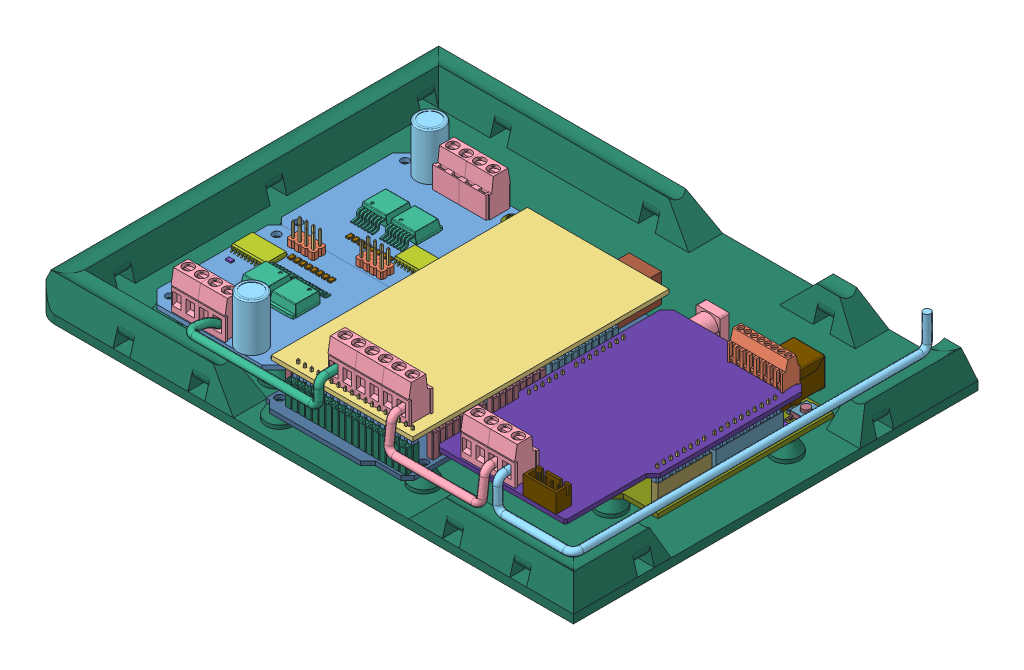
SolidWorks assembly electronics_tray, configuration Default. Lengths in mm.
Overall size (203.2 36.13 152.4).
275 component instances, 60 part files, 29 mates.
Components (placement in the parent):
- ibt2_assembly-1: ibt2_assembly [Default] at (25.1982 40.7289 22.1019) size (49.66 21.28 49.78)
  - IBT2_pcb-1: IBT2_pcb [Default] at (-57.2691 7.2367 24.7687) size (49.66 1.57 49.4)
  - header_male_2x4-1: header_male_2x4 [Default] at (4.8115 23.0826 24.5335) x (1 0 0) z (0 -1 0) size (10.16 5.08 10.92)
    - header_pin_base_2x4-1: header_pin_base_2x4 [Default] at (-49.9521 21.6346 11.7311) size (10.16 5.08 2.54)
    - header_pin-1: header_pin [Default] at (-56.3021 22.9046 6.0161) size (0.64 0.64 10.92)
    - header_pin-2: header_pin [Default] at (-56.3021 20.3646 6.0161) size (0.64 0.64 10.92)
    - header_pin-3: header_pin [Default] at (-53.7621 22.9046 6.0161) size (0.64 0.64 10.92)
    - header_pin-4: header_pin [Default] at (-53.7621 20.3646 6.0161) size (0.64 0.64 10.92)
    - header_pin-5: header_pin [Default] at (-51.2221 22.9046 6.0161) size (0.64 0.64 10.92)
    - header_pin-6: header_pin [Default] at (-51.2221 20.3646 6.0161) size (0.64 0.64 10.92)
    - header_pin-7: header_pin [Default] at (-48.6821 22.9046 6.0161) size (0.64 0.64 10.92)
    - header_pin-8: header_pin [Default] at (-48.6821 20.3646 6.0161) size (0.64 0.64 10.92)
  - AMP_screw-terminal_2POS_large-1: AMP_screw-terminal_2POS_large [Default] at (-57.2056 17.0115 0.4662) x (-1 0 0) z (0 0 -1) size (10.66 17 9)
  - AMP_screw-terminal_2POS_large-2: AMP_screw-terminal_2POS_large [Default] at (-47.0456 17.0115 0.4662) x (-1 0 0) z (0 0 -1) size (10.66 17 9)
  - cap_5mm_pitch-1: cap_5mm_pitch [Default] at (-68.3924 8.8115 4.7662) size (10.16 19.69 10.16)
  - d2pak-1: d2pak [Default] at (-63.2409 8.7779 25.6248) x (1 0 0) z (0 0.999978 0.006671) size (9.87 15.09 4.26)
  - d2pak-2: d2pak [Default] at (-52.336 8.7779 25.6248) x (1 0 0) z (0 0.999978 0.006671) size (9.87 15.09 4.26)
  - SOIC20 wide-1: SOIC20 wide [Default] at (-39.9304 8.5615 36.0347) x (1 0 0) z (0 1 0) size (13 10.17 2.01)
  - cap_0805-1: cap_0805 [Default] at (-38.0286 9.3449 27.3468) x (1 0 0) z (0 -1 0) size (2.03 1.32 0.56)
  - resistor_0805-1: resistor_0805 [Default] at (-48.3156 9.3449 41.6216) x (0 0 -1) z (0 -1 0) size (2.03 1.32 0.56)
  - resistor_0805-2: resistor_0805 [Default] at (-50.4517 9.3449 41.6216) x (0 0 -1) z (0 -1 0) size (2.03 1.32 0.56)
  - resistor_0805-3: resistor_0805 [Default] at (-52.5879 9.3449 41.6216) x (0 0 -1) z (0 -1 0) size (2.03 1.32 0.56)
  - resistor_0805-4: resistor_0805 [Default] at (-54.724 9.3449 41.6216) x (0 0 -1) z (0 -1 0) size (2.03 1.32 0.56)
  - resistor_0805-5: resistor_0805 [Default] at (-56.8602 9.3449 41.6216) x (0 0 -1) z (0 -1 0) size (2.03 1.32 0.56)
  - resistor_0805-6: resistor_0805 [Default] at (-58.9963 9.3449 41.6216) x (0 0 -1) z (0 -1 0) size (2.03 1.32 0.56)
  - resistor_0805-7: resistor_0805 [Default] at (-61.1324 9.3449 41.6216) x (0 0 -1) z (0 -1 0) size (2.03 1.32 0.56)
  - resistor_0805-8: resistor_0805 [Default] at (-63.2686 9.3449 41.6216) x (0 0 -1) z (0 -1 0) size (2.03 1.32 0.56)
- ibt2_assembly-2: ibt2_assembly [Default] at (-89.34 40.7289 121.0422) x (-1 0 0) z (0 0 -1) size (49.66 21.28 49.78)
  - IBT2_pcb-1: IBT2_pcb [Default] at (-57.2691 7.2367 24.7687) size (49.66 1.57 49.4)
  - header_male_2x4-1: header_male_2x4 [Default] at (4.8115 23.0826 24.5335) x (1 0 0) z (0 -1 0) size (10.16 5.08 10.92)
    - header_pin_base_2x4-1: header_pin_base_2x4 [Default] at (-49.9521 21.6346 11.7311) size (10.16 5.08 2.54)
    - header_pin-1: header_pin [Default] at (-56.3021 22.9046 6.0161) size (0.64 0.64 10.92)
    - header_pin-2: header_pin [Default] at (-56.3021 20.3646 6.0161) size (0.64 0.64 10.92)
    - header_pin-3: header_pin [Default] at (-53.7621 22.9046 6.0161) size (0.64 0.64 10.92)
    - header_pin-4: header_pin [Default] at (-53.7621 20.3646 6.0161) size (0.64 0.64 10.92)
    - header_pin-5: header_pin [Default] at (-51.2221 22.9046 6.0161) size (0.64 0.64 10.92)
    - header_pin-6: header_pin [Default] at (-51.2221 20.3646 6.0161) size (0.64 0.64 10.92)
    - header_pin-7: header_pin [Default] at (-48.6821 22.9046 6.0161) size (0.64 0.64 10.92)
    - header_pin-8: header_pin [Default] at (-48.6821 20.3646 6.0161) size (0.64 0.64 10.92)
  - AMP_screw-terminal_2POS_large-1: AMP_screw-terminal_2POS_large [Default] at (-57.2056 17.0115 0.4662) x (-1 0 0) z (0 0 -1) size (10.66 17 9)
  - AMP_screw-terminal_2POS_large-2: AMP_screw-terminal_2POS_large [Default] at (-47.0456 17.0115 0.4662) x (-1 0 0) z (0 0 -1) size (10.66 17 9)
  - cap_5mm_pitch-1: cap_5mm_pitch [Default] at (-68.3924 8.8115 4.7662) size (10.16 19.69 10.16)
  - d2pak-1: d2pak [Default] at (-63.2409 8.7779 25.6248) x (1 0 0) z (0 0.999978 0.006671) size (9.87 15.09 4.26)
  - d2pak-2: d2pak [Default] at (-52.336 8.7779 25.6248) x (1 0 0) z (0 0.999978 0.006671) size (9.87 15.09 4.26)
  - SOIC20 wide-1: SOIC20 wide [Default] at (-39.9304 8.5615 36.0347) x (1 0 0) z (0 1 0) size (13 10.17 2.01)
  - cap_0805-1: cap_0805 [Default] at (-38.0286 9.3449 27.3468) x (1 0 0) z (0 -1 0) size (2.03 1.32 0.56)
  - resistor_0805-1: resistor_0805 [Default] at (-48.3156 9.3449 41.6216) x (0 0 -1) z (0 -1 0) size (2.03 1.32 0.56)
  - resistor_0805-2: resistor_0805 [Default] at (-50.4517 9.3449 41.6216) x (0 0 -1) z (0 -1 0) size (2.03 1.32 0.56)
  - resistor_0805-3: resistor_0805 [Default] at (-52.5879 9.3449 41.6216) x (0 0 -1) z (0 -1 0) size (2.03 1.32 0.56)
  - resistor_0805-4: resistor_0805 [Default] at (-54.724 9.3449 41.6216) x (0 0 -1) z (0 -1 0) size (2.03 1.32 0.56)
  - resistor_0805-5: resistor_0805 [Default] at (-56.8602 9.3449 41.6216) x (0 0 -1) z (0 -1 0) size (2.03 1.32 0.56)
  - resistor_0805-6: resistor_0805 [Default] at (-58.9963 9.3449 41.6216) x (0 0 -1) z (0 -1 0) size (2.03 1.32 0.56)
  - resistor_0805-7: resistor_0805 [Default] at (-61.1324 9.3449 41.6216) x (0 0 -1) z (0 -1 0) size (2.03 1.32 0.56)
  - resistor_0805-8: resistor_0805 [Default] at (-63.2686 9.3449 41.6216) x (0 0 -1) z (0 -1 0) size (2.03 1.32 0.56)
- Arduino_mega-1: Arduino_mega [Default] at (5.4045 37.4555 130.5264) x (0 0 1) z (0 1 0) size (107.7 53.34 12.38)
  - Arduino_mega-1: Arduino_mega [Default] at (-98.4513 -6.297 10.51) size (101.6 53.34 1.59)
  - USB-jack-1: USB-jack [Default] at (-104.5473 25.6308 12.0975) size (16.46 12.14 10.79)
  - DC-jack-1: DC-jack [Default] at (-99.9245 -2.5632 12.0975) x (0 1 0) z (0 0 -1) size (8.79 13.59 10.72)
  - header_8-pin-1: header_8-pin [Default] at (-53.7727 -5.0778 12.0975) size (20.32 2.54 8.56)
  - header_8-pin-2: header_8-pin [Default] at (-30.6587 -5.0778 12.0975) size (20.32 2.54 8.56)
  - header_8-pin-3: header_8-pin [Default] at (-8.0781 -5.0778 12.0975) size (20.32 2.54 8.56)
  - header_8-pin-4: header_8-pin [Default] at (-35.7895 43.0044 12.0975) size (20.32 2.54 8.56)
  - header_8-pin-5: header_8-pin [Default] at (-13.1835 43.0044 12.0975) size (20.32 2.54 8.56)
  - header_10-pin-1: header_10-pin [Default] at (-58.0145 43.0044 12.0975) size (25.4 2.54 8.56)
  - header_36-pin-1: header_36-pin [Default] at (-0.5343 43.0298 12.0975) x (0 1 0) z (0 0 1) size (45.72 5.08 8.56)
- arduino uno-1: arduino uno [Default] at (57.5276 49.6156 28.9001) x (-1 0 0) z (0 0 -1) size (53.34 15.25 74.97)
  - unoboard blue-1: unoboard blue [Default] at origin size (53.34 1.65 68.58)
  - 47uf CAP Dcase-1: 47uf CAP Dcase [Default] at (-9.4141 0 -18.4991) x (0 0 -1) z (1 0 0) size (6.6 5.81 8)
  - USB type b-1: USB type b [Default] at (-38.02 0.43 6.35) size (14.34 15.2 16.54)
    - USB SHELL-1: USB SHELL [Default] at origin size (14.34 15.2 16.54)
    - USB core-1: USB core [Default] at origin size (11.3 10.68 15.75)
    - usb top contact-1: usb top contact [Default] at (1.25 6.09 -0.38) size (1 9.67 13.76)
    - usb btm contact-1: usb btm contact [Default] at (1.25 4.41 -0.38) size (1 6.84 11.76)
    - usb btm contact-2: usb btm contact [Default] at (-1.25 4.41 -0.38) size (1 6.84 11.76)
    - usb top contact-2: usb top contact [Default] at (-1.25 6.09 -0.38) size (1 9.67 13.76)
  - power jack-1: power jack [Default] at (-7.675 0 1.905) size (11.2 15.2 15.9)
  - 47uf CAP Dcase-2: 47uf CAP Dcase [Default] at (-9.4141 0 -25.7132) x (0 0 -1) z (1 0 0) size (6.6 5.81 8)
  - crystal-1: crystal [Default] at (-26.162 0 -18.923) x (1 0 0) z (0 0 -1) size (4 5 11)
  - 2pin_header__02-1: 2pin_header__02 [Default] at (-46.23 0 -15.75) size (5 11.75 2.54)
  - nano - reg-1: nano - reg [Default] at (-17.399 0 -7.747) size (6.5 1.69 8.3)
  - led-1: led [Default] at (-34.29 0 -27.94) x (0 0 1) z (-1 0 0) size (4 0.86 1.35)
  - 2pin_header__02-2: 2pin_header__02 [Default] at (-30.43 0 -64.91) x (0 0 1) z (-1 0 0) size (5 11.75 2.54)
  - dip28-1: dip28 [Default] at (-16.383 1.5 -46.355) x (0 0 -1) z (1 0 0) size (35.48 7.37 10.1)
    - dip28-1: dip28 [Default] at origin size (35.48 2.8 10.1)
    - dip socket pin-1: dip socket pin [Default] at (16.51 2.8 -3.81) size (1.7 7.37 1.7)
    - dip socket pin-2: dip socket pin [Default] at (16.51 2.8 3.81) size (1.7 7.37 1.7)
    - dip socket pin-3: dip socket pin [Default] at (13.97 2.8 -3.81) size (1.7 7.37 1.7)
    - dip socket pin-4: dip socket pin [Default] at (13.97 2.8 3.81) size (1.7 7.37 1.7)
    - dip socket pin-5: dip socket pin [Default] at (11.43 2.8 -3.81) size (1.7 7.37 1.7)
    - dip socket pin-6: dip socket pin [Default] at (11.43 2.8 3.81) size (1.7 7.37 1.7)
    - dip socket pin-7: dip socket pin [Default] at (8.89 2.8 -3.81) size (1.7 7.37 1.7)
    - dip socket pin-8: dip socket pin [Default] at (8.89 2.8 3.81) size (1.7 7.37 1.7)
    - dip socket pin-9: dip socket pin [Default] at (6.35 2.8 -3.81) size (1.7 7.37 1.7)
    - dip socket pin-10: dip socket pin [Default] at (6.35 2.8 3.81) size (1.7 7.37 1.7)
    - dip socket pin-11: dip socket pin [Default] at (3.81 2.8 -3.81) size (1.7 7.37 1.7)
    - dip socket pin-12: dip socket pin [Default] at (3.81 2.8 3.81) size (1.7 7.37 1.7)
    - dip socket pin-13: dip socket pin [Default] at (1.27 2.8 -3.81) size (1.7 7.37 1.7)
    - dip socket pin-14: dip socket pin [Default] at (1.27 2.8 3.81) size (1.7 7.37 1.7)
    - dip socket pin-15: dip socket pin [Default] at (-1.27 2.8 -3.81) size (1.7 7.37 1.7)
    - dip socket pin-16: dip socket pin [Default] at (-1.27 2.8 3.81) size (1.7 7.37 1.7)
    - dip socket pin-17: dip socket pin [Default] at (-3.81 2.8 -3.81) size (1.7 7.37 1.7)
    - dip socket pin-18: dip socket pin [Default] at (-3.81 2.8 3.81) size (1.7 7.37 1.7)
    - dip socket pin-19: dip socket pin [Default] at (-6.35 2.8 -3.81) size (1.7 7.37 1.7)
    - dip socket pin-20: dip socket pin [Default] at (-6.35 2.8 3.81) size (1.7 7.37 1.7)
    - dip socket pin-21: dip socket pin [Default] at (-8.89 2.8 -3.81) size (1.7 7.37 1.7)
    - dip socket pin-22: dip socket pin [Default] at (-8.89 2.8 3.81) size (1.7 7.37 1.7)
    - dip socket pin-23: dip socket pin [Default] at (-11.43 2.8 -3.81) size (1.7 7.37 1.7)
    - dip socket pin-24: dip socket pin [Default] at (-11.43 2.8 3.81) size (1.7 7.37 1.7)
    - dip socket pin-25: dip socket pin [Default] at (-13.97 2.8 -3.81) size (1.7 7.37 1.7)
    - dip socket pin-26: dip socket pin [Default] at (-13.97 2.8 3.81) size (1.7 7.37 1.7)
    - dip socket pin-27: dip socket pin [Default] at (-16.51 2.8 -3.81) size (1.7 7.37 1.7)
    - dip socket pin-28: dip socket pin [Default] at (-16.51 2.8 3.81) size (1.7 7.37 1.7)
  - 2pin_header__02-3: 2pin_header__02 [Default] at (-27.89 0 -64.91) x (0 0 1) z (-1 0 0) size (5 11.75 2.54)
  - 2pin_header__02-4: 2pin_header__02 [Default] at (-25.35 0 -64.91) x (0 0 1) z (-1 0 0) size (5 11.75 2.54)
  - 2pin_header__02-5: 2pin_header__02 [Default] at (-46.23 0 -18.29) size (5 11.75 2.54)
  - 2pin_header__02-6: 2pin_header__02 [Default] at (-46.23 0 -20.83) size (5 11.75 2.54)
  - atmega16u2-1: atmega16u2 [Default] at (-34.671 0.06 -20) x (1 0 0) z (0 0 -1) size (5.5 1.01 5.5)
  - led-2: led [Default] at (-36.83 0 -27.94) x (0 0 1) z (-1 0 0) size (4 0.86 1.35)
  - led-3: led [Default] at (-42.037 0 -27.94) x (0 0 1) z (-1 0 0) size (4 0.86 1.35)
  - led-4: led [Default] at (-36.576 0 -58.42) x (0 0 1) z (-1 0 0) size (4 0.86 1.35)
  - 8 PORT HEADER-3: 8 PORT HEADER [Default] at (-50.8 0 -45.72) x (0 0 -1) z (1 0 0) size (20.32 10.51 2.41)
  - 8 PORT HEADER-4: 8 PORT HEADER [Default] at (-2.54 0 -27.94) x (0 0 -1) z (1 0 0) size (20.32 10.51 2.41)
  - 6 PORT HEADER-3: 6 PORT HEADER [Default] at (-2.54 0 -50.8) x (0 0 -1) z (1 0 0) size (15.24 10.51 2.41)
  - 10 PORT HEADER-1: 10 PORT HEADER [Default] at (-50.8 0 -18.796) x (0 0 -1) z (1 0 0) size (25.4 10.51 2.41)
  - ATMEL328P-1: ATMEL328P [Default] at (-16.383 4.3 -46.355) x (0 0 -1) z (1 0 0) size (35 7.27 7.87)
  - 102 RESISTOR PACK-1: 102 RESISTOR PACK [Default] at (-33.782 0 -58.42) size (3.2 0.46 3)
  - 102 RESISTOR PACK-2: 102 RESISTOR PACK [Default] at (-39.37 0 -27.94) size (3.2 0.46 3)
  - 103 RESISTOR PACK-3: 103 RESISTOR PACK [Default] at (-23.876 0 -27.94) size (3.2 0.46 3)
  - 220 RESISTOR PACK-1: 220 RESISTOR PACK [Default] at (-36.83 0 -12.827) size (3.2 0.46 3)
  - 16mhz crystal - measured-1: 16mhz crystal - measured [Default] at (-24.892 0 -41.275) x (0 0 -1) z (1 0 0) size (3.4 0.8 2)
  - PADS001-1: PADS001 [Default] at (-39.878 0.1 -18.288) x (-1 0 0) z (0 0 1) size (4.54 0.1 4.54)
  - 603 cap on pad-1: 603 cap on pad [Default] at (-44.45 0 -27.94) x (0 0 -1) z (1 0 0) size (2.76 0.9 1.12)
  - ssot3-1: ssot3 [Default] at (-26.5 0 -8.128) x (-1 0 0) z (0 0 -1) size (3 1.13 3.09)
  - mf-msmf050-2-1: mf-msmf050-2 [Default] at (-26.5 0 -4.064) size (5.77 1.02 3.72)
  - 603 cap on pad-2: 603 cap on pad [Default] at (-29.845 0 -27.94) x (0 0 -1) z (1 0 0) size (2.76 0.9 1.12)
  - 603 cap on pad-3: 603 cap on pad [Default] at (-31.496 0 -27.94) x (0 0 -1) z (1 0 0) size (2.76 0.9 1.12)
  - lmv358-1: lmv358 [Default] at (-15.24 0 -21.971) x (0 0 -1) z (1 0 0) size (3.7 1.4 2.9)
  - 603 cap on pad-4: 603 cap on pad [Default] at (-15.24 0 -18.415) size (2.76 0.9 1.12)
  - 603 cap on pad-5: 603 cap on pad [Default] at (-29.845 0 -12.065) x (0 0 1) z (-1 0 0) size (2.76 0.9 1.12)
  - 603 cap on pad-6: 603 cap on pad [Default] at (-29.591 0 -22.352) x (0 0 1) z (-1 0 0) size (2.76 0.9 1.12)
  - 603 cap on pad-7: 603 cap on pad [Default] at (-29.591 0 -16.002) x (0 0 1) z (-1 0 0) size (2.76 0.9 1.12)
  - 603 cap on pad-8: 603 cap on pad [Default] at (-41.91 0 -12.7) x (0 0 1) z (-1 0 0) size (2.76 0.9 1.12)
  - lp2985dgkr-1: lp2985dgkr [Default] at (-20.32 0 -19.05) x (0 0 -1) z (1 0 0) size (5.85 1.1 3)
  - cd1206 diode-1: cd1206 diode [Default] at (-27.94 0 -59.436) x (0 0 -1) z (1 0 0) size (2.07 0.96 5)
  - cd1206 diode-2: cd1206 diode [Default] at (-46.228 0 -13.081) x (0 0 1) z (-1 0 0) size (2.07 0.96 5)
  - 603 resistor-1: 603 resistor [Default] at (-29.591 0 -19.05) x (0 0 1) z (-1 0 0) size (2.36 0.61 1.03)
  - blm21-1: blm21 [Default] at (-45.085 0 -7.62) x (0 0 -1) z (1 0 0) size (2.76 0.95 1.32)
  - m7 diode-1: m7 diode [Default] at (-2.794 0 -21.59) x (0 0 -1) z (1 0 0) size (6.66 2.35 2.5)
  - MLC0603-1: MLC0603 [Default] at (-33.655 0 -12.827) x (0 0 -1) z (1 0 0) size (2.36 0.6 1.03)
  - MLC0603-2: MLC0603 [Default] at (-39.37 0 -12.827) x (0 0 -1) z (1 0 0) size (2.36 0.6 1.03)
  - RESET BUTTON-1: RESET BUTTON [Default] at (-49.403 0 -6.35) size (6.2 3.1 9.6)
    - RESET CORE-1: RESET CORE [Default] at (0 0.1 0) x (-1 0 0) z (0 0 -1) size (6.2 3.1 9.6)
    - RESET-1: RESET [Default] at (0 0.1 0) x (0 0 1) z (-1 0 0) size (7.3 2 6.2)
  - 603 cap on pad-9: 603 cap on pad [Default] at (-15.24 0 -25.625) size (2.76 0.9 1.12)
- electronics_tray_tray-1: electronics_tray_tray [Default] at origin size (203.2 13.95 152.4)
- m3x6mm_cap_screw-1: m3x6mm_cap_screw [92095A179] at (-11.9414 51.1904 27.3507) x (-0.837169 0 -0.546944) z (0 1 0) size (5.7 5.7 7.77)
- bms_assembly-1: bms_assembly [Default] at (83.3041 41.8308 46.3558) x (0 0 -1) z (0 1 0) size (88.9 53.34 22.95)
  - bms_board-1: bms_board [Default] at (-80.72 -27.381 18.8348) size (88.9 53.34 1.57)
  - AMP_screw-terminal_2POS_large-1: AMP_screw-terminal_2POS_large [Default] at (-79.94 10.719 28.6096) x (0 -1 0) z (-1 0 0) size (10.66 17 9)
  - AMP_screw-terminal_2POS_large-2: AMP_screw-terminal_2POS_large [Default] at (-79.94 0.559 28.6096) x (0 -1 0) z (-1 0 0) size (10.66 17 9)
  - B4B-XH-Apart-1: B4B-XH-Apart [Default] at (-77.791 -14.995 20.4096) x (0 1 0) z (1 0 0) size (12.4 10.4 5.75)
  - header_male_1x10-1: header_male_1x10 [Default] at (49.0022 32.4877 36.1995) x (0 1 0) z (0 0 1) size (2.54 25.4 10.92)
    - header_pin-1: header_pin [Default] at (-57.3287 73.639 -25.2387) size (0.64 0.64 10.92)
    - header_pin_base_single-1: header_pin_base_single [Default] at (-58.5987 72.369 -19.9047) size (2.54 2.54 2.54)
    - header_pin_base_single-2: header_pin_base_single [Default] at (-58.5987 69.829 -19.9047) size (2.54 2.54 2.54)
    - header_pin_base_single-3: header_pin_base_single [Default] at (-58.5987 67.289 -19.9047) size (2.54 2.54 2.54)
    - header_pin_base_single-4: header_pin_base_single [Default] at (-58.5987 64.749 -19.9047) size (2.54 2.54 2.54)
    - header_pin_base_single-5: header_pin_base_single [Default] at (-58.5987 62.209 -19.9047) size (2.54 2.54 2.54)
    - header_pin_base_single-6: header_pin_base_single [Default] at (-58.5987 59.669 -19.9047) size (2.54 2.54 2.54)
    - header_pin-2: header_pin [Default] at (-57.3287 71.099 -25.2387) size (0.64 0.64 10.92)
    - header_pin-3: header_pin [Default] at (-57.3287 68.559 -25.2387) size (0.64 0.64 10.92)
    - header_pin-4: header_pin [Default] at (-57.3287 66.019 -25.2387) size (0.64 0.64 10.92)
    - header_pin-5: header_pin [Default] at (-57.3287 63.479 -25.2387) size (0.64 0.64 10.92)
    - header_pin-6: header_pin [Default] at (-57.3287 60.939 -25.2387) size (0.64 0.64 10.92)
    - header_pin-7: header_pin [Default] at (-57.3287 58.399 -25.2387) size (0.64 0.64 10.92)
    - header_pin-8: header_pin [Default] at (-57.3287 55.859 -25.2387) size (0.64 0.64 10.92)
    - header_pin_base_single-7: header_pin_base_single [Default] at (-58.5987 57.129 -19.9047) size (2.54 2.54 2.54)
    - header_pin_base_single-8: header_pin_base_single [Default] at (-58.5987 54.589 -19.9047) size (2.54 2.54 2.54)
    - header_pin_base_single-9: header_pin_base_single [Default] at (-58.5987 52.049 -19.9047) size (2.54 2.54 2.54)
    - header_pin_base_single-10: header_pin_base_single [Default] at (-58.5987 49.509 -19.9047) size (2.54 2.54 2.54)
    - header_pin-9: header_pin [Default] at (-57.3287 53.319 -25.2387) size (0.64 0.64 10.92)
    - header_pin-10: header_pin [Default] at (-57.3287 50.779 -25.2387) size (0.64 0.64 10.92)
  - header_male_1x8-1: header_male_1x8 [Default] at (-84.3058 -33.9097 36.1995) x (0 -1 0) z (0 0 1) size (2.54 20.32 10.92)
    - header_pin-1: header_pin [Default] at (-57.3287 73.639 -25.2387) size (0.64 0.64 10.92)
    - header_pin_base_single-1: header_pin_base_single [Default] at (-58.5987 72.369 -19.9047) size (2.54 2.54 2.54)
    - header_pin_base_single-2: header_pin_base_single [Default] at (-58.5987 69.829 -19.9047) size (2.54 2.54 2.54)
    - header_pin_base_single-3: header_pin_base_single [Default] at (-58.5987 67.289 -19.9047) size (2.54 2.54 2.54)
    - header_pin_base_single-4: header_pin_base_single [Default] at (-58.5987 64.749 -19.9047) size (2.54 2.54 2.54)
    - header_pin_base_single-5: header_pin_base_single [Default] at (-58.5987 62.209 -19.9047) size (2.54 2.54 2.54)
    - header_pin_base_single-6: header_pin_base_single [Default] at (-58.5987 59.669 -19.9047) size (2.54 2.54 2.54)
    - header_pin-2: header_pin [Default] at (-57.3287 71.099 -25.2387) size (0.64 0.64 10.92)
    - header_pin-3: header_pin [Default] at (-57.3287 68.559 -25.2387) size (0.64 0.64 10.92)
    - header_pin-4: header_pin [Default] at (-57.3287 66.019 -25.2387) size (0.64 0.64 10.92)
    - header_pin-5: header_pin [Default] at (-57.3287 63.479 -25.2387) size (0.64 0.64 10.92)
    - header_pin-6: header_pin [Default] at (-57.3287 60.939 -25.2387) size (0.64 0.64 10.92)
    - header_pin-7: header_pin [Default] at (-57.3287 58.399 -25.2387) size (0.64 0.64 10.92)
    - header_pin-8: header_pin [Default] at (-57.3287 55.859 -25.2387) size (0.64 0.64 10.92)
    - header_pin_base_single-7: header_pin_base_single [Default] at (-58.5987 57.129 -19.9047) size (2.54 2.54 2.54)
    - header_pin_base_single-8: header_pin_base_single [Default] at (-58.5987 54.589 -19.9047) size (2.54 2.54 2.54)
  - header_male_1x8-2: header_male_1x8 [Default] at (-102.0858 -82.1697 36.1995) x (0 -1 0) z (0 0 1) size (2.54 20.32 10.92)
    - header_pin-1: header_pin [Default] at (-57.3287 73.639 -25.2387) size (0.64 0.64 10.92)
    - header_pin_base_single-1: header_pin_base_single [Default] at (-58.5987 72.369 -19.9047) size (2.54 2.54 2.54)
    - header_pin_base_single-2: header_pin_base_single [Default] at (-58.5987 69.829 -19.9047) size (2.54 2.54 2.54)
    - header_pin_base_single-3: header_pin_base_single [Default] at (-58.5987 67.289 -19.9047) size (2.54 2.54 2.54)
    - header_pin_base_single-4: header_pin_base_single [Default] at (-58.5987 64.749 -19.9047) size (2.54 2.54 2.54)
    - header_pin_base_single-5: header_pin_base_single [Default] at (-58.5987 62.209 -19.9047) size (2.54 2.54 2.54)
    - header_pin_base_single-6: header_pin_base_single [Default] at (-58.5987 59.669 -19.9047) size (2.54 2.54 2.54)
    - header_pin-2: header_pin [Default] at (-57.3287 71.099 -25.2387) size (0.64 0.64 10.92)
    - header_pin-3: header_pin [Default] at (-57.3287 68.559 -25.2387) size (0.64 0.64 10.92)
    - header_pin-4: header_pin [Default] at (-57.3287 66.019 -25.2387) size (0.64 0.64 10.92)
    - header_pin-5: header_pin [Default] at (-57.3287 63.479 -25.2387) size (0.64 0.64 10.92)
    - header_pin-6: header_pin [Default] at (-57.3287 60.939 -25.2387) size (0.64 0.64 10.92)
    - header_pin-7: header_pin [Default] at (-57.3287 58.399 -25.2387) size (0.64 0.64 10.92)
    - header_pin-8: header_pin [Default] at (-57.3287 55.859 -25.2387) size (0.64 0.64 10.92)
    - header_pin_base_single-7: header_pin_base_single [Default] at (-58.5987 57.129 -19.9047) size (2.54 2.54 2.54)
    - header_pin_base_single-8: header_pin_base_single [Default] at (-58.5987 54.589 -19.9047) size (2.54 2.54 2.54)
  - header_male_1x6-1: header_male_1x6 [Default] at (27.4122 80.7477 36.1995) x (0 1 0) z (0 0 1) size (2.54 15.24 10.92)
    - header_pin-1: header_pin [Default] at (-57.3287 73.639 -25.2387) size (0.64 0.64 10.92)
    - header_pin_base_single-1: header_pin_base_single [Default] at (-58.5987 72.369 -19.9047) size (2.54 2.54 2.54)
    - header_pin_base_single-2: header_pin_base_single [Default] at (-58.5987 69.829 -19.9047) size (2.54 2.54 2.54)
    - header_pin_base_single-3: header_pin_base_single [Default] at (-58.5987 67.289 -19.9047) size (2.54 2.54 2.54)
    - header_pin_base_single-4: header_pin_base_single [Default] at (-58.5987 64.749 -19.9047) size (2.54 2.54 2.54)
    - header_pin_base_single-5: header_pin_base_single [Default] at (-58.5987 62.209 -19.9047) size (2.54 2.54 2.54)
    - header_pin_base_single-6: header_pin_base_single [Default] at (-58.5987 59.669 -19.9047) size (2.54 2.54 2.54)
    - header_pin-2: header_pin [Default] at (-57.3287 71.099 -25.2387) size (0.64 0.64 10.92)
    - header_pin-3: header_pin [Default] at (-57.3287 68.559 -25.2387) size (0.64 0.64 10.92)
    - header_pin-4: header_pin [Default] at (-57.3287 66.019 -25.2387) size (0.64 0.64 10.92)
    - header_pin-5: header_pin [Default] at (-57.3287 63.479 -25.2387) size (0.64 0.64 10.92)
    - header_pin-6: header_pin [Default] at (-57.3287 60.939 -25.2387) size (0.64 0.64 10.92)
  - AMP_screw-terminal_8POS_small-1: AMP_screw-terminal_8POS_small [Default] at (4.7256 -13.9952 30.4096) x (0 1 0) z (0 0 1) size (20.78 6.55 13.4)
- mainboard_assembly-1: mainboard_assembly [Default] at (75.8522 66.1104 104.8773) size (53.34 22.95 96.52)
  - AMP_screw-terminal_2POS_large-1: AMP_screw-terminal_2POS_large [Default] at (-33.2598 4.3173 21.1598) size (10.66 17 9)
  - mainboard_pcb-1: mainboard_pcb [Default] at (-23.6078 -5.4575 23.8448) x (0 0 -1) z (1 0 0) size (96.52 1.57 53.34)
  - AMP_screw-terminal_2POS_large-2: AMP_screw-terminal_2POS_large [Default] at (-53.5798 4.3173 21.1598) size (10.66 17 9)
  - AMP_screw-terminal_2POS_large-3: AMP_screw-terminal_2POS_large [Default] at (-43.4198 4.3173 21.1598) size (10.66 17 9)
  - header_male_1x18-1: header_male_1x18 [Default] at (4.3112 11.9071 -36.0239) x (0 0 -1) z (0 1 0) size (2.54 45.72 10.92)
    - header_pin-1: header_pin [Default] at (-57.3287 73.639 -25.2387) size (0.64 0.64 10.92)
    - header_pin_base_single-1: header_pin_base_single [Default] at (-58.5987 72.369 -19.9047) size (2.54 2.54 2.54)
    - header_pin_base_single-2: header_pin_base_single [Default] at (-58.5987 69.829 -19.9047) size (2.54 2.54 2.54)
    - header_pin_base_single-3: header_pin_base_single [Default] at (-58.5987 67.289 -19.9047) size (2.54 2.54 2.54)
    - header_pin_base_single-4: header_pin_base_single [Default] at (-58.5987 64.749 -19.9047) size (2.54 2.54 2.54)
    - header_pin_base_single-5: header_pin_base_single [Default] at (-58.5987 62.209 -19.9047) size (2.54 2.54 2.54)
    - header_pin_base_single-6: header_pin_base_single [Default] at (-58.5987 59.669 -19.9047) size (2.54 2.54 2.54)
    - header_pin-2: header_pin [Default] at (-57.3287 71.099 -25.2387) size (0.64 0.64 10.92)
    - header_pin-3: header_pin [Default] at (-57.3287 68.559 -25.2387) size (0.64 0.64 10.92)
    - header_pin-4: header_pin [Default] at (-57.3287 66.019 -25.2387) size (0.64 0.64 10.92)
    - header_pin-5: header_pin [Default] at (-57.3287 63.479 -25.2387) size (0.64 0.64 10.92)
    - header_pin-6: header_pin [Default] at (-57.3287 60.939 -25.2387) size (0.64 0.64 10.92)
    - header_pin-7: header_pin [Default] at (-57.3287 58.399 -25.2387) size (0.64 0.64 10.92)
    - header_pin-8: header_pin [Default] at (-57.3287 55.859 -25.2387) size (0.64 0.64 10.92)
    - header_pin_base_single-7: header_pin_base_single [Default] at (-58.5987 57.129 -19.9047) size (2.54 2.54 2.54)
    - header_pin_base_single-8: header_pin_base_single [Default] at (-58.5987 54.589 -19.9047) size (2.54 2.54 2.54)
    - header_pin_base_single-9: header_pin_base_single [Default] at (-58.5987 52.049 -19.9047) size (2.54 2.54 2.54)
    - header_pin_base_single-10: header_pin_base_single [Default] at (-58.5987 49.509 -19.9047) size (2.54 2.54 2.54)
    - header_pin-9: header_pin [Default] at (-57.3287 53.319 -25.2387) size (0.64 0.64 10.92)
    - header_pin-10: header_pin [Default] at (-57.3287 50.779 -25.2387) size (0.64 0.64 10.92)
    - header_pin-11: header_pin [Default] at (-57.3287 48.239 -25.2387) size (0.64 0.64 10.92)
    - header_pin-12: header_pin [Default] at (-57.3287 45.699 -25.2387) size (0.64 0.64 10.92)
    - header_pin-13: header_pin [Default] at (-57.3287 43.159 -25.2387) size (0.64 0.64 10.92)
    - header_pin-14: header_pin [Default] at (-57.3287 40.619 -25.2387) size (0.64 0.64 10.92)
    - header_pin-15: header_pin [Default] at (-57.3287 38.079 -25.2387) size (0.64 0.64 10.92)
    - header_pin-16: header_pin [Default] at (-57.3287 35.539 -25.2387) size (0.64 0.64 10.92)
    - header_pin-17: header_pin [Default] at (-57.3287 32.999 -25.2387) size (0.64 0.64 10.92)
    - header_pin-18: header_pin [Default] at (-57.3287 30.459 -25.2387) size (0.64 0.64 10.92)
    - header_pin_base_single-11: header_pin_base_single [Default] at (-58.5987 46.969 -19.9047) size (2.54 2.54 2.54)
    - header_pin_base_single-12: header_pin_base_single [Default] at (-58.5987 44.429 -19.9047) size (2.54 2.54 2.54)
    - header_pin_base_single-13: header_pin_base_single [Default] at (-58.5987 41.889 -19.9047) size (2.54 2.54 2.54)
    - header_pin_base_single-14: header_pin_base_single [Default] at (-58.5987 39.349 -19.9047) size (2.54 2.54 2.54)
    - header_pin_base_single-15: header_pin_base_single [Default] at (-58.5987 36.809 -19.9047) size (2.54 2.54 2.54)
    - header_pin_base_single-16: header_pin_base_single [Default] at (-58.5987 34.269 -19.9047) size (2.54 2.54 2.54)
    - header_pin_base_single-17: header_pin_base_single [Default] at (-58.5987 31.729 -19.9047) size (2.54 2.54 2.54)
    - header_pin_base_single-18: header_pin_base_single [Default] at (-58.5987 29.189 -19.9047) size (2.54 2.54 2.54)
- wire_gnd-bms-main^electronics_tray-1: wire_gnd-bms-main^electronics_tray [Default] at (0 50.7851 -6.0475) x (1 -0.000001 -0.000005) z (0 0.992984 -0.118245) size (37.87 6.32 15) (virtual)
- wire_gnd-bms-battery^electronics_tray-1: wire_gnd-bms-battery^electronics_tray [Default] at (82.7451 70.4404 124.8958) size (31.16 14.04 136.17) (virtual)
- wire_gnd-main-BTS^electronics_tray-1: wire_gnd-main-BTS^electronics_tray [Default] at (22.2724 70.4277 124.6371) size (52.12 15.48 13.93) (virtual)
Mates (geometry in assembly coordinates):
- Coincident1: coincident anti-aligned: plane of ibt2_assembly-1/IBT2_pcb-1 through (-56.8994 49.5404 71.5721) normal (0 0 1); plane of ibt2_assembly-2/IBT2_pcb-1 through (-7.2424 49.5404 71.5721) normal (0 0 -1)
- Coincident2: coincident aligned: plane of ibt2_assembly-1/IBT2_pcb-1 through (-7.2424 49.5404 71.5721) normal (1 0 0); plane of ibt2_assembly-2/IBT2_pcb-1 through (-7.2424 49.5404 71.5721) normal (1 0 0)
- Coincident3: coincident aligned: plane of ibt2_assembly-1/IBT2_pcb-1 through (-32.0709 47.9656 46.8706) normal (0 -1 0); plane of ibt2_assembly-2/IBT2_pcb-1 through (-32.0709 47.9656 96.2736) normal (0 -1 0)
- Coincident4: coincident aligned: plane of ibt2_assembly-2/IBT2_pcb-1 through (-32.0709 47.9656 96.2736) normal (0 -1 0); plane of Arduino_mega-1/Arduino_mega-1 through (-0.8924 47.9656 32.0751) normal (0 -1 0)
- Distance1: distance = 6.35 mm anti-aligned: plane of ibt2_assembly-1/IBT2_pcb-1 through (-7.2424 49.5404 71.5721) normal (1 0 0); plane of Arduino_mega-1/Arduino_mega-1 through (-0.8924 49.5531 32.0751) normal (-1 0 0)
- Distance2: distance = 12.7 mm aligned: plane of ibt2_assembly-2/IBT2_pcb-1 through (-7.2424 49.5404 120.9751) normal (0 0 1); plane of Arduino_mega-1/Arduino_mega-1 through (-0.8924 49.5531 133.6751) normal (0 0 1)
- Coincident7: coincident aligned: plane of Arduino_mega-1/Arduino_mega-1 through (-0.8924 47.9656 32.0751) normal (0 -1 0); plane of arduino uno-1/unoboard blue-1 through (57.5276 47.9656 28.9001) normal (0 -1 0)
- Coincident11: coincident anti-aligned: plane of ibt2_assembly-1/IBT2_pcb-1 through (-32.0709 49.5404 46.8706) normal (0 1 0); plane of m3x6mm_cap_screw-1 through (-10.3826 49.5404 24.9648) normal (0 -1 0)
- Concentric1: concentric aligned: cylinder of ibt2_assembly-1/IBT2_pcb-1 through (-11.9414 47.9656 27.3507) axis (0 1 0) radius 1.5; line of m3x6mm_cap_screw-1 through (-11.9414 43.5404 27.3507) axis (0 1 0)
- Distance3: distance = 44.45 mm aligned: plane of arduino uno-1/unoboard blue-1 through (57.5276 47.9656 28.9001) normal (0 0 -1); plane of electronics_tray_tray-1 through (120.9006 42.784 -15.5499) normal (0 0 -1)
- Parallel5: parallel aligned: plane of arduino uno-1/unoboard blue-1 through (57.5276 47.9656 28.9001) normal (0 0 -1); plane of bms_assembly-1/bms_board-1 through (59.8851 62.2404 38.1758) normal (0 0 -1)
- Coincident17: coincident anti-aligned: plane of arduino uno-1/6 PORT HEADER-3 through (60.0676 58.1256 79.7001) normal (0 1 0); plane of bms_assembly-1/header_male_1x6-1/header_pin_base_single-1 through (61.1551 58.1256 91.3126) normal (0 -1 0)
- Coincident20: coincident anti-aligned: line of arduino uno-1/6 PORT HEADER-3 through (59.5676 53.1256 92.9001) axis (0 1 0); line of bms_assembly-1/header_male_1x6-1/header_pin-1 through (59.5676 63.2736 92.9001) axis (0 -1 0)
- Distance4: distance = 5.08 mm anti-aligned: plane of arduino uno-1/unoboard blue-1 through (57.5276 47.9656 28.9001) normal (-1 0 0); plane of Arduino_mega-1/Arduino_mega-1 through (52.4476 49.5531 32.0751) normal (1 0 0)
- Coincident22: coincident anti-aligned: plane of Arduino_mega-1/header_36-pin-1 through (48.4344 58.1129 129.9921) normal (0 1 0); plane of mainboard_assembly-1/header_male_1x18-1/header_pin_base_single-18 through (50.9744 58.1129 127.4521) normal (0 -1 0)
- Parallel6: parallel aligned: plane of Arduino_mega-1/Arduino_mega-1 through (-0.8924 49.5531 133.6751) normal (0 0 1); plane of mainboard_assembly-1/mainboard_pcb-1 through (52.2444 62.2277 128.7221) normal (0 0 1)
- Coincident24: coincident anti-aligned: line of Arduino_mega-1/header_36-pin-1 through (6.2069 51.7629 126.4996) axis (0 1 0); line of mainboard_assembly-1/header_male_1x18-1/header_pin-1 through (6.2069 63.2609 126.4996) axis (0 -1 0)
- InPlace1: in place: plane of ? through (0 50.7851 -6.0475) normal (0 0.992984 -0.118245); moOrthogonalPlaneRef_w of ? through (0 50.7851 -6.0475) normal (0 -0.118245 -0.992984); unknown of ?; unknown of wire_gnd-bms-main^electronics_tray-1
- Coincident25: coincident aligned: plane of wire_gnd-bms-main^electronics_tray-1; plane of assembly
- Coincident26: coincident aligned: plane of wire_gnd-bms-main^electronics_tray-1; moOrthogonalPlaneRef_w of assembly
- Coincident27: coincident anti-aligned: plane of wire_gnd-bms-main^electronics_tray-1; moOrthogonalPlaneRef_w of assembly
- InPlace2: in place: plane of bms_assembly-1/AMP_screw-terminal_2POS_large-2 through (82.7451 70.4404 124.8958) normal (0 0 1); plane of ? through (0 0 124.8958) normal (0 0 1); plane of bms_assembly-1/AMP_screw-terminal_2POS_large-2 through (82.7451 70.4404 124.8958) normal (0 0 1); plane of ? through (0 0 124.8958) normal (0 1 0); plane of bms_assembly-1/AMP_screw-terminal_2POS_large-2 through (82.7451 70.4404 124.8958) normal (0 0 1); plane of ? through (0 0 124.8958) normal (1 0 0); plane of bms_assembly-1/AMP_screw-terminal_2POS_large-2 through (82.7451 70.4404 124.8958) normal (0 0 1); unknown of wire_gnd-bms-battery^electronics_tray-1
- Coincident25: coincident aligned: plane of ?; plane of wire_gnd-bms-battery^electronics_tray-1
- Coincident26: coincident aligned: moOrthogonalPlaneRef_w of bms_assembly-1/AMP_screw-terminal_2POS_large-2 through (82.7451 70.4404 124.8958) normal (0 1 0); plane of wire_gnd-bms-battery^electronics_tray-1 through (82.7451 70.4404 124.8958) normal (0 1 0)
- Coincident27: coincident anti-aligned: moOrthogonalPlaneRef_w of bms_assembly-1/AMP_screw-terminal_2POS_large-2 through (82.7451 70.4404 124.8958) normal (-1 0 0); plane of wire_gnd-bms-battery^electronics_tray-1 through (82.7451 70.4404 124.8958) normal (1 0 0)
- InPlace3: in place: plane of mainboard_assembly-1/AMP_screw-terminal_2POS_large-2 through (22.2724 70.4277 124.6371) normal (0 0 1); plane of ? through (0 0 124.6371) normal (0 0 1); plane of mainboard_assembly-1/AMP_screw-terminal_2POS_large-2 through (22.2724 70.4277 124.6371) normal (0 0 1); plane of ? through (0 0 124.6371) normal (0 1 0); plane of mainboard_assembly-1/AMP_screw-terminal_2POS_large-2 through (22.2724 70.4277 124.6371) normal (0 0 1); plane of ? through (0 0 124.6371) normal (1 0 0); plane of mainboard_assembly-1/AMP_screw-terminal_2POS_large-2 through (22.2724 70.4277 124.6371) normal (0 0 1); unknown of wire_gnd-main-BTS^electronics_tray-1
- Coincident28: coincident aligned: plane of ?; plane of wire_gnd-main-BTS^electronics_tray-1
- Coincident29: coincident aligned: moOrthogonalPlaneRef_w of mainboard_assembly-1/AMP_screw-terminal_2POS_large-2 through (22.2724 70.4277 124.6371) normal (0 1 0); plane of wire_gnd-main-BTS^electronics_tray-1 through (22.2724 70.4277 124.6371) normal (0 1 0)
- Coincident30: coincident anti-aligned: moOrthogonalPlaneRef_w of mainboard_assembly-1/AMP_screw-terminal_2POS_large-2 through (22.2724 70.4277 124.6371) normal (-1 0 0); plane of wire_gnd-main-BTS^electronics_tray-1 through (22.2724 70.4277 124.6371) normal (1 0 0)
